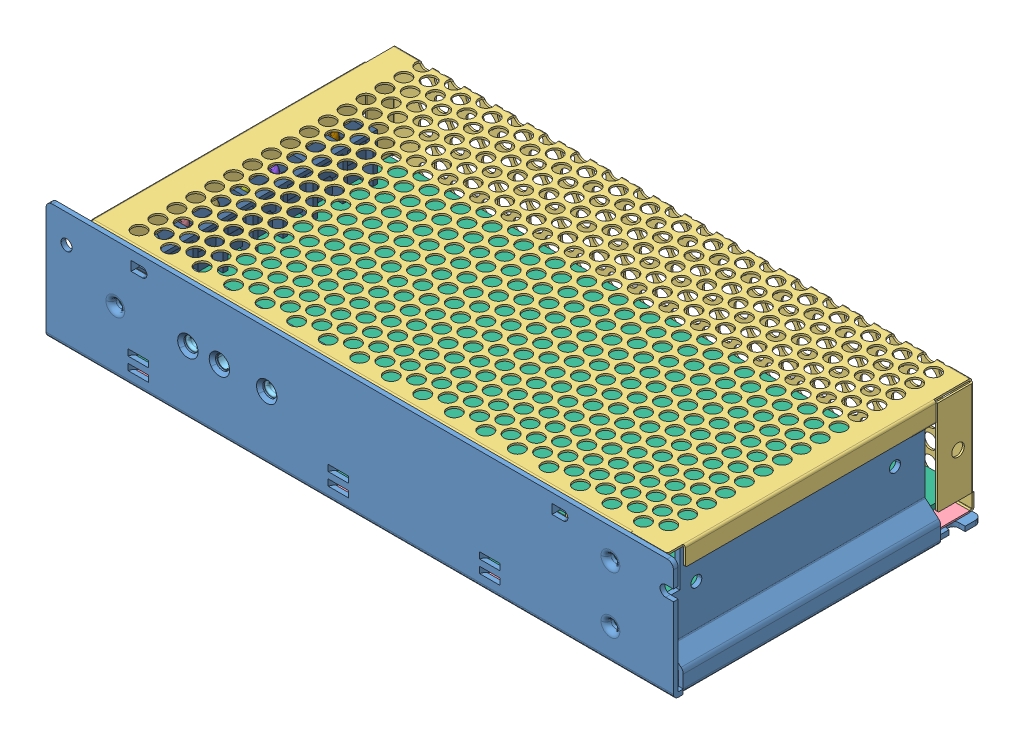
SolidWorks assembly SD-100C-12, configuration Default. Lengths in mm.
Overall size (199.09 37.75 98.27).
20 component instances, 14 part files, 0 mates.
Components (placement in the parent):
- SD-100C-12.stp-1: SD-100C-12.stp [Default] at origin size (199.09 37.75 98.27)
  - SD-100-20201028.stp.stp-1: SD-100-20201028.stp.stp [Default] at origin size (199.09 37.75 98.27)
    - SD-100_STP.ASM.stp-1: SD-100_STP.ASM.stp [Default] at origin size (199.09 37.75 98.27)
      - SD-100_1_ASM.ASM.stp-1: SD-100_1_ASM.ASM.stp [Default] at origin size (199 37.75 98.27)
        - 902-D-80_ASM.ASM.stp-1: 902-D-80_ASM.ASM.stp [Default] at origin size (199 37.75 97.75)
          - 902-D-119_PRT.PRT.stp-1: 902-D-119_PRT.PRT.stp [Default] at origin size (199 37.75 97.75)
          - NUT_PRT.PRT.stp-1: NUT_PRT.PRT.stp [Default] at (-111.528 -1.5 -40.7894) x (-1 0 0) z (0 1 0) size (8 6.93 6)
        - 902-T_PRT.PRT.stp-1: 902-T_PRT.PRT.stp [Default] at (96.5 36.1 -49.375) x (-1 0 0) z (0 0 -1) size (195.5 36.02 96.52)
        - MYLAR_PRT.PRT.stp-1: MYLAR_PRT.PRT.stp [Default] at (79.2081 1.5 46.5396) x (-1 0 0) z (0 -1 0) size (197 95 0.5)
        - HS2_PRT.PRT.stp-1: HS2_PRT.PRT.stp [Default] at (-64.5 -80.2586 -88.3567) x (0 0 1) z (-1 0 0) size (6.4 28 55)
        - PCB_PRT.PRT.stp-1: PCB_PRT.PRT.stp [Default] at (-189.5595 4.5 45.0362) x (1 0 0) z (0 1 0) size (194 95 1.6)
      - T44-BS1R05370120201023_STP.ASM.stp-1: T44-BS1R05370120201023_STP.ASM.stp [Default] at (-82.3888 6.1 -32.875) x (0 0 1) z (0 1 0) size (69.8 18 18.8)
        - 6_PRT.PRT.stp-1: 6_PRT.PRT.stp [Default] at origin size (7.51 7.5 3.96)
        - 2_PRT.PRT.stp-1: 2_PRT.PRT.stp [Default] at origin size (7.5 7.5 3.96)
        - 3_PRT.PRT.stp-1: 3_PRT.PRT.stp [Default] at origin size (7.51 7.5 3.96)
        - 4_PRT.PRT.stp-1: 4_PRT.PRT.stp [Default] at (0 0.8 0) size (69.8 18 18.8)
        - 5_PRT.PRT.stp-1: 5_PRT.PRT.stp [Default] at origin size (7.51 7.5 3.96)
        - 6_PRT_1.PRT.stp-1: 6_PRT_1.PRT.stp [Default] at (9.5 0 0) size (7.51 7.5 3.96)
        - 6_PRT_1_1.PRT.stp-1: 6_PRT_1_1.PRT.stp [Default] at (19 0 0) size (7.51 7.5 3.96)
        - 6_PRT_1_1_1.PRT.stp-1: 6_PRT_1_1_1.PRT.stp [Default] at (28.5 0 0) size (7.51 7.5 3.96)
